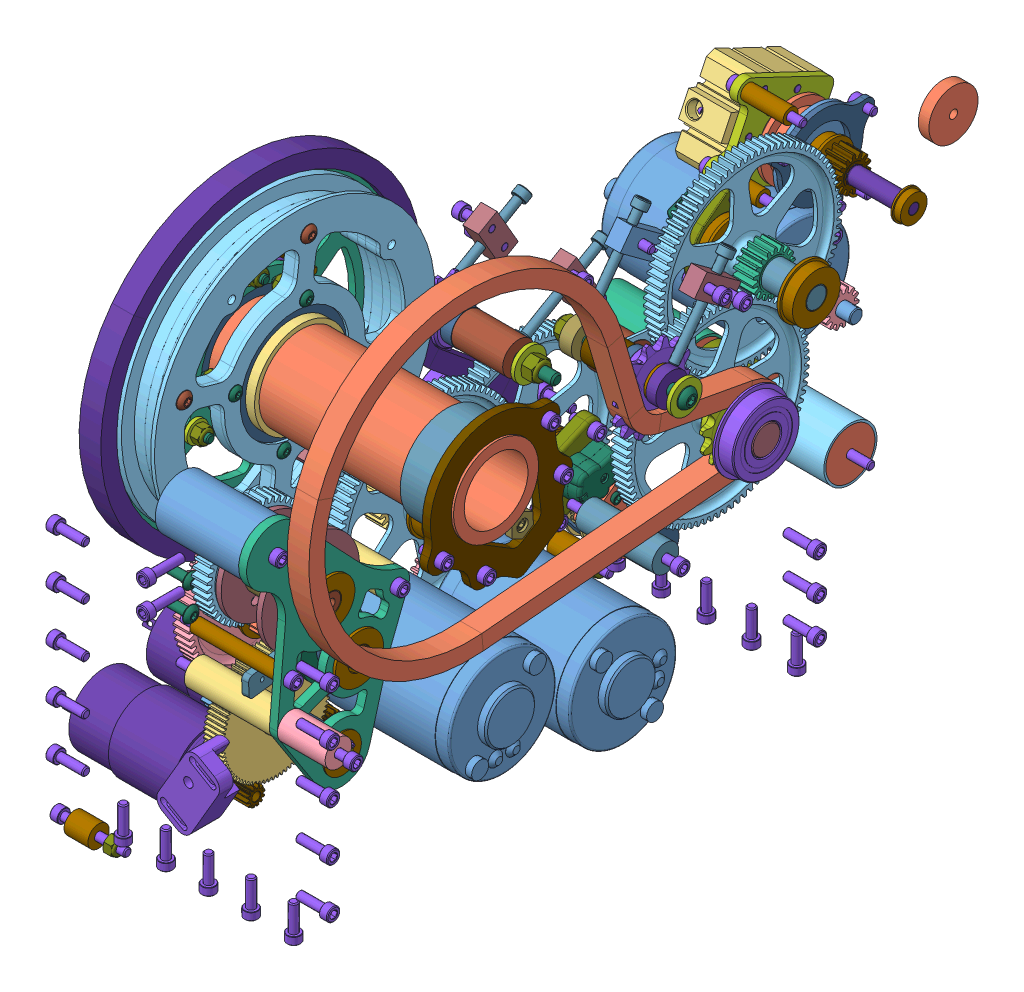
SolidWorks assembly 971-18-A-2900_Arm Gearbox, configuration Default. Lengths in mm. (continued)
Mates (geometry in assembly coordinates): (continued)
- Concentric136: concentric aligned: cylinder of 971-18-P-0057_Arm Gearbox Plates-1 through (0 -27.627 -17.6289) axis (-1 0 0) radius 2.0193; cylinder of 84865A130_10-32 Mitebite LOW-PROFILE CLAMP-1 through (-3.5814 -27.627 -17.6289) axis (-1 0 0) radius 2.413
- Coincident139: coincident anti-aligned: plane of 971-18-P-0057_Arm Gearbox Plates-1 through (0 0 0) normal (-1 0 0); plane of 84865A130_10-32 Mitebite LOW-PROFILE CLAMP-1 through (0 -35.3804 -18.2274) normal (1 0 0)
- Parallel1: parallel anti-aligned: plane of 971-18-P-0101_Tensioner Strap-1 through (-4.7625 -29.9915 -25.9171) normal (0 0.842996 0.537919); plane of 84865A130_10-32 Mitebite LOW-PROFILE CLAMP-1 through (-4.064 -31.4362 -24.4085) normal (0 -0.842996 -0.537919)
- Concentric137: concentric anti-aligned: cylinder of 971-18-P-0057_Arm Gearbox Plates-1 through (0 -27.627 -17.6289) axis (-1 0 0) radius 2.0193; cylinder of 84865A130_10-32 Mitebite LOW-PROFILE CLAMP-2 through (162.3314 -27.627 -17.6289) axis (1 0 0) radius 2.413
- Coincident141: coincident anti-aligned: plane of 971-18-P-0057_Arm Gearbox Plates-1 through (158.75 0 0) normal (1 0 0); plane of 84865A130_10-32 Mitebite LOW-PROFILE CLAMP-2 through (158.75 -31.4362 -24.4085) normal (-1 0 0)
- Parallel2: parallel anti-aligned: plane of 971-18-P-0101_Tensioner Strap-2 through (158.75 -29.9915 -25.9171) normal (0 0.842996 0.537919); plane of 84865A130_10-32 Mitebite LOW-PROFILE CLAMP-2 through (162.814 -35.3804 -18.2274) normal (0 -0.842996 -0.537919)
- Concentric138: concentric anti-aligned: cylinder of 971-18-P-0104_Arm Gearbox Proximal Arm Output Shaft-1 through (161.22 -58.42 -165.2367) axis (-1 0 0) radius 6.35; cylinder of 1_2in Shaft Collar, 217-2736-1 through (94.8323 -58.42 -165.2367) axis (1 0 0) radius 6.477
- Concentric140: concentric anti-aligned: cylinder of 971-18-P-0057_Arm Gearbox Plates-1 through (101.9302 42.553 -239.0191) axis (-1 0 0) radius 2.0193; cylinder of 971-18-A-4900_Brake Assembly-1/971-18-P-0165_Brake Piston Mount-1 through (71.628 42.553 -239.0191) axis (1 0 0) radius 6.35
- Concentric141: concentric aligned: cylinder of 971-18-P-0057_Arm Gearbox Plates-1 through (101.9302 24.3862 -284.3456) axis (-1 0 0) radius 2.0193; cylinder of 971-18-P-0148_Brake Pad-1 through (101.9302 24.3862 -284.3456) axis (-1 0 0) radius 2.4892
- Concentric142: concentric anti-aligned: cylinder of 971-18-P-0148_Brake Pad-1 through (101.9302 24.3862 -284.3456) axis (-1 0 0) radius 2.4892; cylinder of SHCS-2 through (98.7552 24.3862 -284.3456) axis (1 0 0) radius 2.413
- Coincident143: coincident anti-aligned: plane of 971-18-P-0148_Brake Pad-1 through (98.7552 27.1024 -246.9922) normal (-1 0 0); plane of SHCS-2 through (98.7552 28.0884 -283.9713) normal (1 0 0)
- Concentric143: concentric aligned: cylinder of 971-18-P-0057_Arm Gearbox Plates-1 through (106.6927 -24.2127 -256.9444) axis (1 0 0) radius 2.4892; cylinder of MiniCIM-1 through (101.9302 -24.2127 -256.9444) axis (1 0 0) radius 2.0193
- Coincident144: coincident anti-aligned: plane of 971-18-P-0057_Arm Gearbox Plates-1 through (106.6927 0 0) normal (1 0 0); plane of SHCS-5 through (106.6927 -23.145 -260.509) normal (-1 0 0)
- Concentric144: concentric anti-aligned: cylinder of 971-18-P-0057_Arm Gearbox Plates-1 through (106.6927 -24.2127 -256.9444) axis (1 0 0) radius 2.4892; cylinder of SHCS-5 through (106.6927 -24.2127 -256.9444) axis (-1 0 0) radius 2.413
- Concentric145: concentric anti-aligned: cylinder of 971-18-P-0057_Arm Gearbox Plates-1 through (106.6927 -66.0952 -228.1956) axis (1 0 0) radius 2.4892; cylinder of SHCS-6 through (106.6927 -66.0952 -228.1956) axis (-1 0 0) radius 2.413
- Coincident145: coincident anti-aligned: plane of 971-18-P-0057_Arm Gearbox Plates-1 through (106.6927 0 0) normal (1 0 0); plane of SHCS-6 through (106.6927 -65.0275 -231.7603) normal (-1 0 0)
- Concentric146: concentric aligned: cylinder of 971-18-P-0057_Arm Gearbox Plates-1 through (63.5 -146.0373 -33.9901) axis (-1 0 0) radius 2.4892; cylinder of MiniCIM-2 through (68.2625 -146.0373 -33.9901) axis (-1 0 0) radius 2.0193
- Concentric147: concentric aligned: cylinder of 971-18-P-0057_Arm Gearbox Plates-1 through (63.5 -164.4054 -67.0748) axis (-1 0 0) radius 2.4892; cylinder of MiniCIM-3 through (68.2625 -164.4054 -67.0748) axis (-1 0 0) radius 2.0193
- Coincident146: coincident anti-aligned: plane of 971-18-P-0057_Arm Gearbox Plates-1 through (63.5 0 0) normal (-1 0 0); plane of SHCS-7 through (63.5 -115.2256 2.9107) normal (1 0 0)
- Concentric148: concentric anti-aligned: cylinder of 971-18-P-0057_Arm Gearbox Plates-1 through (63.5 -111.5234 3.285) axis (-1 0 0) radius 2.4892; cylinder of SHCS-7 through (63.5 -111.5234 3.285) axis (1 0 0) radius 2.413
- Concentric149: concentric anti-aligned: cylinder of 971-18-P-0116_Arm Proximal Side Spacer-2 through (56.646 45.4322 -285.7008) axis (-1 0 0) radius 15.875; cylinder of 971-18-A-6600_Arm Hard Stop-1/971-18-P-0133_Arm hard stop-1 through (106.6927 45.4322 -285.7008) axis (1 0 0) radius 16.125
- Coincident147: coincident anti-aligned: plane of 971-18-P-0057_Arm Gearbox Plates-1 through (106.6927 0 0) normal (1 0 0); plane of 971-18-A-6600_Arm Hard Stop-1/971-18-P-0133_Arm hard stop-1 through (106.6927 68.5291 -272.3658) normal (-1 0 0)
- Angle1: planar angle = 0.523599 rad aligned: plane of 971-18-A-6600_Arm Hard Stop-1/971-18-P-0133_Arm hard stop-1 through (119.3927 68.5291 -272.3658) normal (0 -0.5 0.866025); plane of assembly through (0 0 0) normal (0 0 1)
- Coincident149: coincident anti-aligned: plane of 971-18-P-0057_Arm Gearbox Plates-1 through (152.4 0 0) normal (-1 0 0); plane of 971-18-P-0116_Arm Proximal Side Spacer-2 through (152.4 47.5844 -301.4292) normal (1 0 0)
- Concentric150: concentric aligned: cylinder of 971-18-P-0057_Arm Gearbox Plates-1 through (0 45.4322 -285.7008) axis (-1 0 0) radius 2.4892; cylinder of 971-18-P-0116_Arm Proximal Side Spacer-2 through (56.646 45.4322 -285.7008) axis (-1 0 0) radius 15.875
- Coincident150: coincident anti-aligned: plane of 971-18-P-0057_Arm Gearbox Plates-1 through (101.9302 0 0) normal (-1 0 0); plane of 971-18-P-0118_Arm Distal Side Double Spacer-1 through (101.9302 57.9871 -275.9854) normal (1 0 0)
- Concentric151: concentric aligned: cylinder of 971-18-P-0116_Arm Proximal Side Spacer-2 through (56.646 45.4322 -285.7008) axis (-1 0 0) radius 15.875; cylinder of 971-18-P-0118_Arm Distal Side Double Spacer-1 through (-18.7539 45.4322 -285.7008) axis (-1 0 0) radius 15.875
- Coincident151: coincident anti-aligned: plane of 971-18-P-0057_Arm Gearbox Plates-1 through (152.4 0 0) normal (-1 0 0); plane of 971-18-P-0116_Arm Proximal Side Spacer-1 through (152.4 -83.5681 -223.1773) normal (1 0 0)
- Concentric152: concentric aligned: cylinder of 971-18-P-0057_Arm Gearbox Plates-1 through (0 -99.4146 -224.1283) axis (-1 0 0) radius 2.4892; cylinder of 971-18-P-0116_Arm Proximal Side Spacer-1 through (56.646 -99.4146 -224.1283) axis (-1 0 0) radius 15.875
- Coincident152: coincident anti-aligned: plane of 971-18-P-0057_Arm Gearbox Plates-1 through (101.9302 0 0) normal (-1 0 0); plane of 971-18-P-0130_Arm Middle Spacer-1 through (101.9302 -100.3998 -239.9727) normal (1 0 0)
- Coincident153: coincident anti-aligned: plane of 971-18-P-0057_Arm Gearbox Plates-1 through (63.5 0 0) normal (-1 0 0); plane of 971-18-P-0115_Arm Distal Side Spacer-1 through (63.5 -85.5318 -216.4287) normal (1 0 0)
- Concentric153: concentric aligned: cylinder of 971-18-P-0057_Arm Gearbox Plates-1 through (0 -99.4146 -224.1283) axis (-1 0 0) radius 2.4892; cylinder of 971-18-P-0115_Arm Distal Side Spacer-1 through (-37.969 -99.4146 -224.1283) axis (-1 0 0) radius 15.875
- Concentric154: concentric aligned: cylinder of 971-18-P-0057_Arm Gearbox Plates-1 through (0 -166.289 -43.6572) axis (-1 0 0) radius 2.4892; cylinder of 971-18-P-0115_Arm Distal Side Spacer-2 through (-37.969 -166.289 -43.6572) axis (-1 0 0) radius 15.875
- Coincident154: coincident anti-aligned: plane of 971-18-P-0057_Arm Gearbox Plates-1 through (63.5 0 0) normal (-1 0 0); plane of 971-18-P-0115_Arm Distal Side Spacer-2 through (63.5 -173.1907 -29.361) normal (1 0 0)
- Concentric157: concentric anti-aligned: cylinder of 971-18-P-0057_Arm Gearbox Plates-1 through (101.9302 -98.1413 -113.6751) axis (-1 0 0) radius 2.4892; cylinder of 971-18-P-0185_Arm cross small standoff-1 through (153.5805 -98.1413 -113.6751) axis (1 0 0) radius 7.9375
- Coincident157: coincident anti-aligned: plane of 971-18-P-0057_Arm Gearbox Plates-1 through (106.6927 0 0) normal (1 0 0); plane of 971-18-P-0185_Arm cross small standoff-1 through (106.6927 -90.2038 -113.6751) normal (-1 0 0)
- Coincident158: coincident anti-aligned: plane of 3549S-1BA-102B-ND 10 turn potentiometer-1 through (66.775 -149.8585 -169.7731) normal (-1 0 0); plane of A-6z16-036df2508_36t plastic pulley-1 through (66.775 -149.8585 -169.7731) normal (1 0 0)
- Coincident166: coincident anti-aligned: plane of SRK Mag Encoder Magnet-2 through (107.2515 -2.1568 -197.4778) normal (1 0 0); plane of 971-18-P-0105_Arm Gearbox Proximal Arm First Stage Shaft -1 through (107.2515 -2.1568 -197.4778) normal (-1 0 0)
- Concentric1943: concentric aligned: cylinder of 971-18-P-0186_84T Gear With Access Hole-1 through (49.3125 -103.4997 -135.089) axis (-1 0 0) radius 8.89; cylinder of 971-18-P-0107_Arm Gearbox Distal Arm Output Shaft-1 through (69.8627 -103.4997 -135.089) axis (-1 0 0) radius 9.525
- Coincident214: coincident anti-aligned: plane of 971-18-P-0186_84T Gear With Access Hole-3 through (121.1339 -2.1568 -197.4778) normal (1 0 0); plane of 18T-1_2-Hex-Steel_217-5460-2 through (121.1339 -2.1568 -197.4778) normal (-1 0 0)
- Concentric1951: concentric anti-aligned: cylinder of 971-18-P-0116_Arm Proximal Side Spacer-1 through (56.646 -99.4146 -224.1283) axis (-1 0 0) radius 14.6304; cylinder of 971-18-P-0229_Arm Spacer Caps-1 through (100.1102 -99.4146 -224.1283) axis (1 0 0) radius 14.6685
- Coincident222: coincident aligned: plane of 971-18-P-0115_Arm Distal Side Spacer-1 through (6.35 -85.5318 -216.4287) normal (-1 0 0); plane of 971-18-P-0229_Arm Spacer Caps-1 through (6.35 -114.0127 -225.5645) normal (-1 0 0)
- Concentric1952: concentric anti-aligned: cylinder of 971-18-P-0116_Arm Proximal Side Spacer-1 through (56.646 -99.4146 -224.1283) axis (-1 0 0) radius 14.6304; cylinder of 971-18-P-0229_Arm Spacer Caps-7 through (150.9102 -99.4146 -224.1283) axis (1 0 0) radius 14.6685
- Coincident223: coincident aligned: plane of 971-18-P-0115_Arm Distal Side Spacer-1 through (63.5 -85.5318 -216.4287) normal (1 0 0); plane of 971-18-P-0229_Arm Spacer Caps-7 through (63.5 -86.8108 -216.6244) normal (1 0 0)
- Concentric1955: concentric anti-aligned: cylinder of 971-18-P-0130_Arm Middle Spacer-1 through (12.196 -99.4146 -224.1283) axis (-1 0 0) radius 14.6304; cylinder of 971-18-P-0229_Arm Spacer Caps-3 through (162.01 -99.4146 -224.1283) axis (1 0 0) radius 14.6685
- Coincident225: coincident aligned: plane of 971-18-P-0130_Arm Middle Spacer-1 through (68.2498 -100.3998 -239.9727) normal (-1 0 0); plane of 971-18-P-0229_Arm Spacer Caps-3 through (68.2498 -113.7159 -220.8666) normal (-1 0 0)
- Concentric1956: concentric aligned: cylinder of 971-18-P-0130_Arm Middle Spacer-1 through (12.196 -99.4146 -224.1283) axis (-1 0 0) radius 14.6304; cylinder of 971-18-P-0229_Arm Spacer Caps-5 through (8.17 -99.4146 -224.1283) axis (-1 0 0) radius 14.6685
- Coincident227: coincident aligned: plane of 971-18-P-0130_Arm Middle Spacer-1 through (101.9302 -100.3998 -239.9727) normal (1 0 0); plane of 971-18-P-0229_Arm Spacer Caps-5 through (101.9302 -84.7547 -224.6303) normal (1 0 0)
- Concentric1958: concentric anti-aligned: cylinder of 971-18-P-0116_Arm Proximal Side Spacer-1 through (56.646 -99.4146 -224.1283) axis (-1 0 0) radius 14.6304; cylinder of 971-18-P-0229_Arm Spacer Caps-2 through (200.4402 -99.4146 -224.1283) axis (1 0 0) radius 14.6685
- Coincident229: coincident aligned: plane of 971-18-P-0116_Arm Proximal Side Spacer-1 through (106.68 -83.5681 -223.1773) normal (-1 0 0); plane of 971-18-P-0229_Arm Spacer Caps-2 through (106.68 -114.0287 -222.8661) normal (-1 0 0)
- Coincident233: coincident aligned: plane of 971-18-P-0116_Arm Proximal Side Spacer-1 through (152.4 -83.5681 -223.1773) normal (1 0 0); plane of 971-18-P-0229_Arm Spacer Caps-6 through (152.4 -114.0831 -224.1283) normal (1 0 0)
- Concentric1962: concentric anti-aligned: cylinder of 971-18-P-0116_Arm Proximal Side Spacer-1 through (56.646 -99.4146 -224.1283) axis (-1 0 0) radius 14.6304; cylinder of 971-18-P-0229_Arm Spacer Caps-6 through (239.8102 -99.4146 -224.1283) axis (1 0 0) radius 14.6685
- Concentric1963: concentric anti-aligned: cylinder of 971-18-P-0115_Arm Distal Side Spacer-2 through (-37.969 -166.289 -43.6572) axis (-1 0 0) radius 14.6304; cylinder of 971-18-P-0229_Arm Spacer Caps-4 through (100.1102 -166.289 -43.6572) axis (1 0 0) radius 14.6685
- Coincident234: coincident aligned: plane of 971-18-P-0115_Arm Distal Side Spacer-2 through (6.35 -173.1907 -29.361) normal (-1 0 0); plane of 971-18-P-0229_Arm Spacer Caps-4 through (6.35 -179.1054 -50.7921) normal (-1 0 0)
- Concentric1964: concentric anti-aligned: cylinder of 971-18-P-0115_Arm Distal Side Spacer-2 through (-37.969 -166.289 -43.6572) axis (-1 0 0) radius 14.6304; cylinder of 971-18-P-0229_Arm Spacer Caps-8 through (150.9102 -166.289 -43.6572) axis (1 0 0) radius 14.6685
- Coincident235: coincident aligned: plane of 971-18-P-0115_Arm Distal Side Spacer-2 through (63.5 -173.1907 -29.361) normal (1 0 0); plane of 971-18-P-0229_Arm Spacer Caps-8 through (63.5 -180.9575 -43.6572) normal (1 0 0)
- Concentric1967: concentric anti-aligned: cylinder of 971-18-P-0057_Arm Gearbox Plates-1 through (0 45.4322 -285.7008) axis (-1 0 0) radius 2.4892; cylinder of SHCS-1 through (0 45.4322 -285.7008) axis (1 0 0) radius 2.413
- Coincident238: coincident anti-aligned: plane of 971-18-P-0057_Arm Gearbox Plates-1 through (0 0 0) normal (-1 0 0); plane of SHCS-1 through (0 42.6322 -283.2499) normal (1 0 0)
- Concentric1968: concentric anti-aligned: cylinder of 971-18-P-0116_Arm Proximal Side Spacer-2 through (56.646 45.4322 -285.7008) axis (-1 0 0) radius 14.6304; cylinder of 971-18-P-0229_Arm Spacer Caps-11 through (239.8102 45.4322 -285.7008) axis (1 0 0) radius 14.6685
- Coincident239: coincident anti-aligned: plane of 971-18-P-0057_Arm Gearbox Plates-1 through (152.4 0 0) normal (-1 0 0); plane of 971-18-P-0229_Arm Spacer Caps-11 through (152.4 30.7637 -285.7008) normal (1 0 0)
- Concentric1969: concentric aligned: cylinder of 971-18-P-0116_Arm Proximal Side Spacer-2 through (56.646 45.4322 -285.7008) axis (-1 0 0) radius 14.6304; cylinder of 971-18-P-0229_Arm Spacer Caps-12 through (19.2825 45.4322 -285.7008) axis (-1 0 0) radius 14.6685
- Coincident240: coincident anti-aligned: plane of 971-18-P-0057_Arm Gearbox Plates-1 through (106.6927 0 0) normal (1 0 0); plane of 971-18-P-0229_Arm Spacer Caps-12 through (106.6927 48.813 -299.9744) normal (-1 0 0)
- Concentric1970: concentric anti-aligned: cylinder of 971-18-P-0116_Arm Proximal Side Spacer-2 through (56.646 45.4322 -285.7008) axis (-1 0 0) radius 14.6304; cylinder of 971-18-P-0229_Arm Spacer Caps-13 through (189.3404 45.4322 -285.7008) axis (1 0 0) radius 14.6685
- Coincident241: coincident anti-aligned: plane of 971-18-P-0057_Arm Gearbox Plates-1 through (101.9302 0 0) normal (-1 0 0); plane of 971-18-P-0229_Arm Spacer Caps-13 through (101.9302 31.3632 -289.8518) normal (1 0 0)
- Concentric1971: concentric aligned: cylinder of 971-18-P-0116_Arm Proximal Side Spacer-2 through (56.646 45.4322 -285.7008) axis (-1 0 0) radius 14.6304; cylinder of 971-18-P-0229_Arm Spacer Caps-14 through (-81.0602 45.4322 -285.7008) axis (-1 0 0) radius 14.6685
- Coincident242: coincident anti-aligned: plane of 971-18-P-0057_Arm Gearbox Plates-1 through (6.35 0 0) normal (1 0 0); plane of 971-18-P-0229_Arm Spacer Caps-14 through (6.35 45.6015 -300.3683) normal (-1 0 0)
- Concentric1973: concentric anti-aligned: cylinder of 971-18-P-0057_Arm Gearbox Plates-1 through (0 -99.4146 -224.1283) axis (-1 0 0) radius 2.4892; cylinder of SHCS-13 through (0 -99.4146 -224.1283) axis (1 0 0) radius 2.413
- Coincident243: coincident anti-aligned: plane of 971-18-P-0057_Arm Gearbox Plates-1 through (0 0 0) normal (-1 0 0); plane of SHCS-13 through (0 -102.1778 -221.636) normal (1 0 0)
- Concentric1974: concentric anti-aligned: cylinder of 971-18-P-0057_Arm Gearbox Plates-1 through (0 -166.289 -43.6572) axis (-1 0 0) radius 2.4892; cylinder of SHCS-14 through (0 -166.289 -43.6572) axis (1 0 0) radius 2.413
- Coincident244: coincident anti-aligned: plane of 971-18-P-0057_Arm Gearbox Plates-1 through (0 0 0) normal (-1 0 0); plane of SHCS-14 through (0 -169.0522 -41.1649) normal (1 0 0)
- Concentric1975: concentric aligned: cylinder of 971-18-P-0057_Arm Gearbox Plates-1 through (101.9302 -98.1413 -113.6751) axis (-1 0 0) radius 2.4892; cylinder of SHCS-16 through (158.75 -98.1413 -113.6751) axis (-1 0 0) radius 2.413
- Coincident245: coincident anti-aligned: plane of 971-18-P-0057_Arm Gearbox Plates-1 through (158.75 0 0) normal (1 0 0); plane of SHCS-16 through (158.75 -97.4126 -117.3241) normal (-1 0 0)
- Concentric1979: concentric anti-aligned: cylinder of Bearings-5 through (98.4246 -2.1568 -197.4778) axis (-1 0 0) radius 14.2875; cylinder of 971-18-A-5400_SRX Mag Encoder 15 Assembly-1/971-18-P-0205_SRX Mag Encoder 15 Mount-3 through (99.7712 -2.1568 -197.4778) axis (1 0 0) radius 14.3002
- Coincident248: coincident anti-aligned: plane of 971-18-P-0057_Arm Gearbox Plates-1 through (101.9302 0 0) normal (-1 0 0); plane of 971-18-A-5400_SRX Mag Encoder 15 Assembly-1/971-18-P-0205_SRX Mag Encoder 15 Mount-3 through (101.9302 -2.1568 -197.4778) normal (1 0 0)
- Concentric1981: concentric anti-aligned: cylinder of 971-18-P-0057_Arm Gearbox Plates-1 through (101.9302 17.5344 -204.6448) axis (-1 0 0) radius 2.0193; cylinder of 971-18-A-5400_SRX Mag Encoder 15 Assembly-1/SHCS-2 through (93.9927 17.5344 -204.6448) axis (1 0 0) radius 2.413
- Concentric1982: concentric anti-aligned: cylinder of Bearings-1 through (71.7681 -103.4997 -135.089) axis (1 0 0) radius 14.2875; cylinder of 971-18-A-5400_SRX Mag Encoder 15 Assembly-2/971-18-P-0205_SRX Mag Encoder 15 Mount-3 through (70.4215 -103.4997 -135.089) axis (-1 0 0) radius 14.3002
- Coincident249: coincident anti-aligned: plane of 971-18-P-0057_Arm Gearbox Plates-1 through (68.2625 0 0) normal (1 0 0); plane of 971-18-A-5400_SRX Mag Encoder 15 Assembly-2/971-18-P-0205_SRX Mag Encoder 15 Mount-3 through (68.2625 -103.4997 -135.089) normal (-1 0 0)
- Concentric1983: concentric anti-aligned: cylinder of 971-18-P-0057_Arm Gearbox Plates-1 through (68.2625 -120.9185 -123.44) axis (1 0 0) radius 2.0193; cylinder of 971-18-A-5400_SRX Mag Encoder 15 Assembly-2/SHCS-1 through (76.2 -120.9185 -123.44) axis (-1 0 0) radius 2.413
- Concentric1984: concentric aligned: cylinder of 971-18-P-0101_Tensioner Strap-2 through (158.75 20.3652 -31.9152) axis (-1 0 0) radius 2.5527; cylinder of SHCS-19 through (163.5125 20.3652 -31.9152) axis (-1 0 0) radius 2.413
- Coincident250: coincident anti-aligned: plane of 971-18-P-0101_Tensioner Strap-2 through (163.5125 0 0) normal (1 0 0); plane of SHCS-19 through (163.5125 24.0861 -31.9561) normal (-1 0 0)
- Concentric1985: concentric anti-aligned: cylinder of 971-18-P-0101_Tensioner Strap-1 through (-4.7625 -20.3652 31.9152) axis (-1 0 0) radius 2.5527; cylinder of SHCS-23 through (-4.7625 -20.3652 31.9152) axis (1 0 0) radius 2.413
- Coincident252: coincident anti-aligned: plane of 971-18-P-0101_Tensioner Strap-1 through (-4.7625 0 0) normal (-1 0 0); plane of SHCS-23 through (-4.7625 -16.968 33.4336) normal (1 0 0)
- Concentric1988: concentric anti-aligned: cylinder of 971-18-P-0057_Arm Gearbox Plates-1 through (158.75 -172.339 95.6183) axis (1 0 0) radius 2.4892; cylinder of SHCS-27 through (158.75 -172.339 95.6183) axis (-1 0 0) radius 2.413
- Coincident255: coincident anti-aligned: plane of 971-18-P-0057_Arm Gearbox Plates-1 through (158.75 0 0) normal (1 0 0); plane of SHCS-27 through (158.75 -169.0333 93.9099) normal (-1 0 0)
- Concentric1989: concentric aligned: cylinder of 971-18-P-0057_Arm Gearbox Plates-1 through (158.75 -172.339 95.6183) axis (1 0 0) radius 2.4892; cylinder of SHCS-28 through (0 -172.339 95.6183) axis (1 0 0) radius 2.413
- Coincident256: coincident anti-aligned: plane of 971-18-P-0057_Arm Gearbox Plates-1 through (0 0 0) normal (-1 0 0); plane of SHCS-28 through (0 -169.5759 93.126) normal (1 0 0)
- Concentric1990: concentric anti-aligned: cylinder of 971-18-P-0057_Arm Gearbox Plates-1 through (158.75 -175.26 -195.2625) axis (1 0 0) radius 2.4892; cylinder of SHCS-37 through (158.75 -175.26 -195.2625) axis (-1 0 0) radius 2.413
- Coincident257: coincident anti-aligned: plane of 971-18-P-0057_Arm Gearbox Plates-1 through (158.75 0 0) normal (1 0 0); plane of SHCS-37 through (158.75 -171.9014 -196.8646) normal (-1 0 0)
- Concentric1991: concentric aligned: cylinder of 971-18-P-0057_Arm Gearbox Plates-1 through (158.75 -175.26 -195.2625) axis (1 0 0) radius 2.4892; cylinder of SHCS-38 through (0 -175.26 -195.2625) axis (1 0 0) radius 2.413
- Coincident258: coincident anti-aligned: plane of 971-18-P-0057_Arm Gearbox Plates-1 through (0 0 0) normal (-1 0 0); plane of SHCS-38 through (0 -172.4969 -197.7548) normal (1 0 0)
- Concentric1995: concentric anti-aligned: cylinder of 971-18-P-0057_Arm Gearbox Plates-1 through (139.6577 -188.214 95.6183) axis (0 -1 0) radius 2.0193; cylinder of SHCS-46 through (139.6577 -192.9892 95.6183) axis (0 1 0) radius 2.413
- Distance1: distance = 4.7752 mm anti-aligned: plane of 971-18-P-0057_Arm Gearbox Plates-1 through (152.4 -188.214 90.8558) normal (0 -1 0); plane of SHCS-46 through (143.3668 -192.9892 95.3205) normal (0 1 0)
- Concentric1996: concentric anti-aligned: cylinder of 971-18-P-0057_Arm Gearbox Plates-1 through (114.2153 -188.214 95.6183) axis (0 -1 0) radius 2.0193; cylinder of SHCS-47 through (114.2153 -192.9892 95.6183) axis (0 1 0) radius 2.413
- Coincident264: coincident aligned: plane of SHCS-46 through (143.3668 -192.9892 95.3205) normal (0 1 0); plane of SHCS-47 through (117.9245 -192.9892 95.3205) normal (0 1 0)
- Concentric1997: concentric anti-aligned: cylinder of 971-18-P-0057_Arm Gearbox Plates-1 through (88.773 -188.214 95.6183) axis (0 -1 0) radius 2.0193; cylinder of SHCS-48 through (88.773 -192.9892 95.6183) axis (0 1 0) radius 2.413
- Coincident265: coincident aligned: plane of SHCS-46 through (143.3668 -192.9892 95.3205) normal (0 1 0); plane of SHCS-48 through (92.3596 -192.9892 94.6268) normal (0 1 0)
- Coincident266: coincident aligned: plane of SHCS-46 through (143.3668 -192.9892 95.3205) normal (0 1 0); plane of SHCS-49 through (66.6192 -192.9892 93.8769) normal (0 1 0)
- Concentric1998: concentric anti-aligned: cylinder of 971-18-P-0057_Arm Gearbox Plates-1 through (63.3307 -188.214 95.6183) axis (0 -1 0) radius 2.0193; cylinder of SHCS-49 through (63.3307 -192.9892 95.6183) axis (0 1 0) radius 2.413
- Coincident267: coincident aligned: plane of SHCS-46 through (143.3668 -192.9892 95.3205) normal (0 1 0); plane of SHCS-50 through (40.677 -192.9892 93.1545) normal (0 1 0)
- Concentric1999: concentric anti-aligned: cylinder of 971-18-P-0057_Arm Gearbox Plates-1 through (37.8883 -188.214 95.6183) axis (0 -1 0) radius 2.0193; cylinder of SHCS-50 through (37.8883 -192.9892 95.6183) axis (0 1 0) radius 2.413
- Concentric2000: concentric anti-aligned: cylinder of 971-18-P-0057_Arm Gearbox Plates-1 through (122.2375 -190.5 -195.2625) axis (0 -1 0) radius 2.0193; cylinder of SHCS-52 through (122.2375 -194.437 -195.2625) axis (0 1 0) radius 2.413
- Distance2: distance = 3.937 mm anti-aligned: plane of 971-18-P-0057_Arm Gearbox Plates-1 through (152.4 -190.5 -200.025) normal (0 -1 0); plane of SHCS-52 through (125.9467 -194.437 -195.5603) normal (0 1 0)
- Concentric2001: concentric anti-aligned: cylinder of 971-18-P-0057_Arm Gearbox Plates-1 through (95.25 -190.5 -195.2625) axis (0 -1 0) radius 2.0193; cylinder of SHCS-53 through (95.25 -194.437 -195.2625) axis (0 1 0) radius 2.413
- Coincident270: coincident aligned: plane of SHCS-52 through (125.9467 -194.437 -195.5603) normal (0 1 0); plane of SHCS-53 through (98.9592 -194.437 -195.5603) normal (0 1 0)
- Coincident271: coincident aligned: plane of SHCS-52 through (125.9467 -194.437 -195.5603) normal (0 1 0); plane of SHCS-54 through (152.8116 -194.437 -196.254) normal (0 1 0)
- Concentric2002: concentric anti-aligned: cylinder of 971-18-P-0057_Arm Gearbox Plates-1 through (149.225 -190.5 -195.2625) axis (0 -1 0) radius 2.0193; cylinder of SHCS-54 through (149.225 -194.437 -195.2625) axis (0 1 0) radius 2.413
- Coincident272: coincident aligned: plane of SHCS-52 through (125.9467 -194.437 -195.5603) normal (0 1 0); plane of SHCS-55 through (71.551 -194.437 -197.0039) normal (0 1 0)
- Concentric2003: concentric anti-aligned: cylinder of 971-18-P-0057_Arm Gearbox Plates-1 through (68.2625 -190.5 -195.2625) axis (0 -1 0) radius 2.0193; cylinder of SHCS-55 through (68.2625 -194.437 -195.2625) axis (0 1 0) radius 2.413
- Coincident273: coincident aligned: plane of SHCS-52 through (125.9467 -194.437 -195.5603) normal (0 1 0); plane of SHCS-56 through (44.0636 -194.437 -197.7263) normal (0 1 0)
- Concentric2004: concentric anti-aligned: cylinder of 971-18-P-0057_Arm Gearbox Plates-1 through (41.275 -190.5 -195.2625) axis (0 -1 0) radius 2.0193; cylinder of SHCS-56 through (41.275 -194.437 -195.2625) axis (0 1 0) radius 2.413
- Coincident278: coincident anti-aligned: plane of 971-18-P-0057_Arm Gearbox Plates-1 through (0 0 0) normal (-1 0 0); plane of SHCS-61 through (0 -205.8981 -198.6843) normal (1 0 0)
- Concentric2009: concentric anti-aligned: cylinder of 971-18-P-0057_Arm Gearbox Plates-1 through (0 -204.4065 -195.2752) axis (-1 0 0) radius 2.4892; cylinder of SHCS-61 through (0 -204.4065 -195.2752) axis (1 0 0) radius 2.413
- Coincident284: coincident anti-aligned: plane of 971-18-P-0057_Arm Gearbox Plates-1 through (6.35 0 0) normal (1 0 0); plane of No 10 Aluminum Spacer-8 through (6.35 -203.0692 -189.0676) normal (-1 0 0)
- Concentric2016: concentric aligned: cylinder of SHCS-61 through (0 -204.4065 -195.2752) axis (1 0 0) radius 2.413; cylinder of No 10 Aluminum Spacer-8 through (56.9589 -204.4065 -195.2752) axis (1 0 0) radius 6.35
- Concentric2020: concentric aligned: cylinder of 971-18-P-0124_Sketchy Chain Tensioner-1 through (15.875 -12.5246 -146.6125) axis (1 0 0) radius 2.0193; cylinder of SHCS-65 through (0 -12.5246 -146.6125) axis (1 0 0) radius 2.413
- Concentric2021: concentric aligned: cylinder of 971-18-P-0124_Sketchy Chain Tensioner-1 through (15.875 -25.7229 -154.2325) axis (1 0 0) radius 2.0193; cylinder of SHCS-67 through (0 -25.7229 -154.2325) axis (1 0 0) radius 2.413
- Concentric2022: concentric aligned: cylinder of 971-18-P-0264_Swoopy thing 2-1 through (101.9302 21.0025 -150.0962) axis (1 0 0) radius 2.4892; cylinder of SHCS-69 through (92.4052 21.0025 -150.0962) axis (1 0 0) radius 2.413
- Coincident291: coincident anti-aligned: plane of 971-18-P-0264_Swoopy thing 2-1 through (92.4052 24.7667 -144.9822) normal (-1 0 0); plane of SHCS-69 through (92.4052 17.8262 -148.1577) normal (1 0 0)
- Concentric2023: concentric aligned: cylinder of 971-18-P-0264_Swoopy thing 2-1 through (101.9302 13.4742 -160.3243) axis (1 0 0) radius 2.4892; cylinder of SHCS-71 through (92.4052 13.4742 -160.3243) axis (1 0 0) radius 2.413
- Coincident292: coincident anti-aligned: plane of 971-18-P-0264_Swoopy thing 2-1 through (92.4052 24.7667 -144.9822) normal (-1 0 0); plane of SHCS-71 through (92.4052 10.2792 -158.4168) normal (1 0 0)
- Concentric2028: concentric aligned: cylinder of 3547S-1AA-102A-ND 3 Turn Potentiometer Bourns-2 through (90.4741 -58.42 -165.2367) axis (-1 0 0) radius 4.5; cylinder of 971-18-P-0243_Arm Gearbox Potentiometer Mount-2 through (101.9312 -58.42 -165.2367) axis (-1 0 0) radius 5.08
- Coincident296: coincident anti-aligned: plane of 971-18-P-0057_Arm Gearbox Plates-1 through (101.9302 0 0) normal (-1 0 0); plane of 971-18-P-0243_Arm Gearbox Potentiometer Mount-2 through (101.9302 -85.7984 -149.5368) normal (1 0 0)
- Parallel3: parallel aligned: plane of 971-18-P-0057_Arm Gearbox Plates-1 through (158.75 -117.7253 -222.1704) normal (0 -0.994332 0.106322); plane of 971-18-P-0243_Arm Gearbox Potentiometer Mount-2 through (100.4062 -73.1704 -150.8871) normal (0 -0.994332 0.106322)
- Concentric2029: concentric anti-aligned: cylinder of 971-18-P-0186_84T Gear With Access Hole-4 through (121.1339 -58.42 -165.2367) axis (1 0 0) radius 8.89; cylinder of VexPro_Hex Spacers-1 through (121.1339 -58.42 -165.2367) axis (-1 0 0) radius 9.7536
- Coincident297: coincident anti-aligned: plane of 971-18-P-0186_84T Gear With Access Hole-4 through (121.1339 -58.42 -165.2367) normal (-1 0 0); plane of VexPro_Hex Spacers-1 through (121.1339 -58.42 -165.2367) normal (1 0 0)
- Coincident298: coincident anti-aligned: plane of 971-18-P-0057_Arm Gearbox Plates-1 through (0 0 0) normal (-1 0 0); plane of SHCS-65 through (0 -14.681 -143.5799) normal (1 0 0)
- Coincident299: coincident anti-aligned: plane of 971-18-P-0057_Arm Gearbox Plates-1 through (0 0 0) normal (-1 0 0); plane of SHCS-67 through (0 -26.6968 -150.6411) normal (1 0 0)
- Concentric2030: concentric anti-aligned: cylinder of 971-18-P-0057_Arm Gearbox Plates-1 through (158.75 29.2837 -138.8453) axis (1 0 0) radius 2.4892; cylinder of SHCS-76 through (158.75 29.2837 -138.8453) axis (-1 0 0) radius 2.413
- Coincident300: coincident anti-aligned: plane of 971-18-P-0057_Arm Gearbox Plates-1 through (158.75 0 0) normal (1 0 0); plane of SHCS-76 through (158.75 32.7317 -140.2447) normal (-1 0 0)
- Concentric2031: concentric anti-aligned: cylinder of 971-18-P-0057_Arm Gearbox Plates-1 through (158.75 20.2497 -151.119) axis (1 0 0) radius 2.4892; cylinder of SHCS-78 through (158.75 20.2497 -151.119) axis (-1 0 0) radius 2.413
- Coincident301: coincident anti-aligned: plane of 971-18-P-0057_Arm Gearbox Plates-1 through (158.75 0 0) normal (1 0 0); plane of SHCS-78 through (158.75 23.4914 -152.946) normal (-1 0 0)
- Concentric2032: concentric aligned: cylinder of 971-18-P-0057_Arm Gearbox Plates-1 through (0 -12.5246 -146.6125) axis (-1 0 0) radius 2.4892; cylinder of SHCS-80 through (68.2625 -12.5246 -146.6125) axis (-1 0 0) radius 2.413
- Coincident302: coincident anti-aligned: plane of 971-18-P-0057_Arm Gearbox Plates-1 through (68.2625 0 0) normal (1 0 0); plane of SHCS-80 through (68.2625 -10.9765 -149.9963) normal (-1 0 0)
- Concentric2033: concentric aligned: cylinder of 971-18-P-0057_Arm Gearbox Plates-1 through (0 -25.7229 -154.2325) axis (-1 0 0) radius 2.4892; cylinder of SHCS-82 through (68.2625 -25.7229 -154.2325) axis (-1 0 0) radius 2.413
- Coincident303: coincident anti-aligned: plane of 971-18-P-0057_Arm Gearbox Plates-1 through (68.2625 0 0) normal (1 0 0); plane of SHCS-82 through (68.2625 -24.7858 -157.8337) normal (-1 0 0)
- Concentric2034: concentric aligned: cylinder of 971-18-P-0186_84T Gear With Access Hole-1 through (49.3125 -103.4997 -135.089) axis (-1 0 0) radius 8.89; cylinder of VexPro_Hex Spacers-2 through (61.9125 -103.4997 -135.089) axis (-1 0 0) radius 9.7536
- Coincident305: coincident anti-aligned: plane of SRK Mag Encoder Magnet-1 through (63.0047 -103.4997 -135.089) normal (-1 0 0); plane of 971-18-P-0107_Arm Gearbox Distal Arm Output Shaft-1 through (63.0047 -100.5783 -133.8458) normal (1 0 0)
- Coincident306: coincident anti-aligned: plane of Bearings-1 through (61.9125 -89.5132 -138.0061) normal (-1 0 0); plane of VexPro_Hex Spacers-2 through (61.9125 -103.4997 -135.089) normal (1 0 0)
- Concentric2035: concentric aligned: cylinder of 971-18-P-0107_Arm Gearbox Distal Arm Output Shaft-1 through (69.8627 -103.4997 -135.089) axis (-1 0 0) radius 9.525; cylinder of 971-18-P-0254_40T plastic pulley hex-1 through (60.9806 -103.4997 -135.089) axis (-1 0 0) radius 15.113
- Coincident307: coincident anti-aligned: plane of 971-18-P-0186_84T Gear With Access Hole-1 through (49.3125 -103.4997 -135.089) normal (1 0 0); plane of 971-18-P-0254_40T plastic pulley hex-1 through (49.3125 -103.4997 -135.089) normal (-1 0 0)
- Concentric2036: concentric aligned: cylinder of 971-18-P-0107_Arm Gearbox Distal Arm Output Shaft-1 through (69.8627 -103.4997 -135.089) axis (-1 0 0) radius 9.525; cylinder of 971-18-P-0249_Distal Shaft Spacer-1 through (36.4604 -103.4997 -135.089) axis (-1 0 0) radius 9.75
- Coincident308: coincident anti-aligned: plane of 12T_Hex_217-2662-2 through (26.5543 -103.4997 -135.089) normal (1 0 0); plane of 971-18-P-0249_Distal Shaft Spacer-1 through (26.5543 -103.4997 -135.089) normal (-1 0 0)
- Parallel4: parallel anti-aligned: plane of 971-18-P-0057_Arm Gearbox Plates-1 through (158.75 -118.7209 -182.2708) normal (0 -0.800703 -0.599061); plane of 971-18-P-0112_Arm Gearbox Distal Potentiometer Mount-1 through (68.345 -133.0932 -141.5671) normal (0 0.800703 0.599061)
- Parallel5: parallel aligned: plane of potentiometer belt-1 through (51.6937 -103.4997 -135.089) normal (0 0.599061 -0.800703); plane of 971-18-P-0112_Arm Gearbox Distal Potentiometer Mount-1 through (68.345 -118.0672 -161.6507) normal (0 0.599061 -0.800703)
- Coincident311: coincident anti-aligned: plane of 3549S-1BA-102B-ND 10 turn potentiometer-1 through (74.695 -149.8585 -169.7731) normal (-1 0 0); plane of 971-18-P-0112_Arm Gearbox Distal Potentiometer Mount-1 through (74.695 -149.8585 -169.7731) normal (1 0 0)
- Concentric2037: concentric anti-aligned: cylinder of SHCS-61 through (0 -204.4065 -195.2752) axis (1 0 0) radius 2.413; cylinder of Nylon-Insert Locknut-3 through (25.6032 -204.4065 -195.2752) axis (-1 0 0) radius 2.0828
- Distance3: distance = 7.0485 mm anti-aligned: plane of No 10 Aluminum Spacer-8 through (20.6375 -203.0692 -189.0676) normal (1 0 0); plane of Nylon-Insert Locknut-3 through (27.686 -199.3722 -195.5352) normal (-1 0 0)
- Concentric2038: concentric anti-aligned: cylinder of 971-18-P-0057_Arm Gearbox Plates-1 through (68.2625 -128.7803 -15.3525) axis (-1 0 0) radius 9.5631; cylinder of MiniCIM-2 through (68.2625 -128.7803 -15.3525) axis (1 0 0) radius 31.877
- Coincident321: coordinate: point of 971-18-P-0057_Arm Gearbox Plates-1; point of 971-18-A-5700_Winch Gearbox-1/971-18-P-0057_Arm Gearbox Plates-1
- Concentric2047: concentric anti-aligned: cylinder of 971-18-P-0057_Arm Gearbox Plates-1 through (63.5 -51.689 86.0933) axis (1 0 0) radius 2.0193; cylinder of BHCS-3 through (53.975 -51.689 86.0933) axis (-1 0 0) radius 2.413
- Coincident322: coincident anti-aligned: plane of 971-18-P-0057_Arm Gearbox Plates-1 through (68.2625 0 0) normal (1 0 0); plane of BHCS-3 through (68.2625 -48.6377 89.5151) normal (-1 0 0)
- Concentric2048: concentric anti-aligned: cylinder of 971-18-P-0057_Arm Gearbox Plates-1 through (63.5 -69.1515 86.0933) axis (1 0 0) radius 2.0193; cylinder of BHCS-4 through (53.975 -69.1515 86.0933) axis (-1 0 0) radius 2.413
- Coincident323: coincident anti-aligned: plane of 971-18-P-0057_Arm Gearbox Plates-1 through (68.2625 0 0) normal (1 0 0); plane of BHCS-4 through (68.2625 -66.1002 89.5151) normal (-1 0 0)
- Concentric2049: concentric anti-aligned: cylinder of 971-18-P-0057_Arm Gearbox Plates-1 through (58.7375 -46.9265 100.3808) axis (0 0 1) radius 2.4892; cylinder of SHCS-88 through (58.7375 -46.9265 100.3808) axis (0 0 -1) radius 2.413
- Concentric2050: concentric anti-aligned: cylinder of 971-18-P-0057_Arm Gearbox Plates-1 through (58.7375 -64.389 100.3808) axis (0 0 1) radius 2.4892; cylinder of SHCS-89 through (58.7375 -64.389 100.3808) axis (0 0 -1) radius 2.413
- Coincident324: coincident anti-aligned: plane of 971-18-P-0057_Arm Gearbox Plates-1 through (152.4 -188.214 100.3808) normal (0 0 1); plane of SHCS-89 through (56.2452 -61.6259 100.3808) normal (0 0 -1)
- Coincident325: coincident anti-aligned: plane of 971-18-P-0057_Arm Gearbox Plates-1 through (152.4 -188.214 100.3808) normal (0 0 1); plane of SHCS-88 through (56.2452 -44.1634 100.3808) normal (0 0 -1)
- Concentric2051: concentric aligned: cylinder of 971-18-P-0057_Arm Gearbox Plates-1 through (63.5 -134.8658 -152.2116) axis (-1 0 0) radius 2.0193; cylinder of BHCS-6 through (61.995 -134.8658 -152.2116) axis (-1 0 0) radius 2.413
- Coincident326: coincident anti-aligned: plane of 971-18-P-0112_Arm Gearbox Distal Potentiometer Mount-1 through (74.695 -149.8585 -169.7731) normal (1 0 0); plane of BHCS-6 through (74.695 -130.8701 -154.4598) normal (-1 0 0)
- Coincident327: coincident anti-aligned: plane of 971-18-P-0112_Arm Gearbox Distal Potentiometer Mount-1 through (74.695 -149.8585 -169.7731) normal (1 0 0); plane of BHCS-7 through (74.695 -124.4777 -161.9329) normal (-1 0 0)
- Concentric2052: concentric aligned: cylinder of 971-18-P-0057_Arm Gearbox Plates-1 through (63.5 -128.7793 -160.3468) axis (-1 0 0) radius 2.0193; cylinder of BHCS-7 through (61.995 -128.7793 -160.3468) axis (-1 0 0) radius 2.413
- Concentric2053: concentric anti-aligned: cylinder of BHCS-1 through (86.614 -39.637 -114.8895) axis (1 0 0) radius 3.175; cylinder of 91525A416_1-4 Oversized Washer-1 through (0 -39.637 -114.8895) axis (-1 0 0) radius 9.525
- Coincident329: coincident anti-aligned: plane of 971-18-P-0057_Arm Gearbox Plates-1 through (0 0 0) normal (-1 0 0); plane of 91525A416_1-4 Oversized Washer-1 through (0 -39.637 -114.8895) normal (1 0 0)
- Concentric2054: concentric aligned: cylinder of 971-18-P-0123_Distal Tensioner Short Spacer-1 through (31.8387 -39.637 -114.8895) axis (1 0 0) radius 3.2639; cylinder of BHCS-1 through (86.614 -39.637 -114.8895) axis (1 0 0) radius 3.175
- Coincident330: coincident anti-aligned: plane of BHCS-1 through (-2.286 -45.1869 -114.8895) normal (1 0 0); plane of 91525A416_1-4 Oversized Washer-1 through (-2.286 -39.637 -114.8895) normal (-1 0 0)
- Concentric2055: concentric anti-aligned: cylinder of BHCS-1 through (86.614 -39.637 -114.8895) axis (1 0 0) radius 3.175; cylinder of 91525A416_1-4 Oversized Washer-2 through (70.5485 -39.637 -114.8895) axis (-1 0 0) radius 3.5687
- Coincident331: coincident anti-aligned: plane of 971-18-P-0057_Arm Gearbox Plates-1 through (68.2625 0 0) normal (1 0 0); plane of 91525A416_1-4 Oversized Washer-2 through (68.2625 -39.637 -114.8895) normal (-1 0 0)
- Coincident332: coincident anti-aligned: plane of Nylon-Insert Locknut-1 through (70.5485 -46.0512 -115.0309) normal (-1 0 0); plane of 91525A416_1-4 Oversized Washer-2 through (70.5485 -39.637 -114.8895) normal (1 0 0)
- Coincident333: coincident anti-aligned: plane of Nylon-Insert Locknut-2 through (94.4372 -11.816 -111.0726) normal (1 0 0); plane of 971-18-P-0123_Distal Tensioner Short Spacer-3 through (94.4372 -5.8623 -110.7598) normal (-1 0 0)
- Concentric2056: concentric aligned: cylinder of BHCS-2 through (84.836 -12.6592 -117.4327) axis (-1 0 0) radius 3.175; cylinder of 91525A416_1-4 Oversized Washer-3 through (161.036 -12.6592 -117.4327) axis (-1 0 0) radius 9.525
- Coincident334: coincident anti-aligned: plane of 971-18-P-0057_Arm Gearbox Plates-1 through (158.75 0 0) normal (1 0 0); plane of 91525A416_1-4 Oversized Washer-3 through (158.75 -12.6592 -117.4327) normal (-1 0 0)
- Concentric2057: concentric anti-aligned: cylinder of 971-18-P-0248_Proximal Tensioner Short Spacer-2 through (171.1668 -12.6592 -117.4327) axis (1 0 0) radius 3.2639; cylinder of BHCS-2 through (84.836 -12.6592 -117.4327) axis (-1 0 0) radius 3.175
- Coincident335: coincident anti-aligned: plane of BHCS-2 through (161.036 -14.7784 -112.3034) normal (-1 0 0); plane of 91525A416_1-4 Oversized Washer-3 through (161.036 -12.6592 -117.4327) normal (1 0 0)
- Coincident336: coincident anti-aligned: plane of SHCS-32 through (163.576 -50.5026 94.0207) normal (1 0 0); plane of 971-18-P-0057_Arm Gearbox Plates-2 through (163.576 -162.56 -197.485) normal (-1 0 0)
- Coincident337: coincident aligned: plane of 971-18-P-0057_Arm Gearbox Plates-1 through (158.75 -188.214 103.5558) normal (0 0 1); plane of 971-18-P-0057_Arm Gearbox Plates-2 through (164.3888 -162.56 103.5558) normal (0 0 1)
- Coincident338: coincident aligned: plane of 971-18-P-0057_Arm Gearbox Plates-1 through (158.75 25.8839 -19.8529) normal (0 0.983523 0.180782); plane of 971-18-P-0057_Arm Gearbox Plates-2 through (164.3888 28.6009 -34.6344) normal (0 0.983523 0.180782)
- Coincident339: coincident aligned: plane of 971-18-P-0057_Arm Gearbox Plates-1 through (158.75 -52.6379 -288.3169) normal (0 -0.161448 -0.986881); plane of 971-18-P-0057_Arm Gearbox Plates-3 through (-5.6388 42.4591 -303.8742) normal (0 -0.161448 -0.986881)
- Coincident340: coincident aligned: plane of 971-18-P-0057_Arm Gearbox Plates-1 through (158.75 25.8839 -19.8529) normal (0 0.989859 0.142055); plane of 971-18-P-0057_Arm Gearbox Plates-3 through (-5.6388 27.324 -29.8876) normal (0 0.989859 0.142055)
- Coincident341: coincident anti-aligned: plane of SHCS-1 through (-4.826 42.8138 -283.4088) normal (-1 0 0); plane of 971-18-P-0057_Arm Gearbox Plates-3 through (-4.826 0 0) normal (1 0 0)
- Coincident344: coincident anti-aligned: plane of 971-18-P-0057_Arm Gearbox Plates-1 through (152.4 -188.214 100.3808) normal (0 0 1); plane of 971-18-P-0352_Arm Gearbox-Bumper Spacer-1 through (90.8758 -115.2621 100.3808) normal (0 0 -1)
- Concentric2061: concentric anti-aligned: cylinder of 971-18-P-0057_Arm Gearbox Plates-1 through (89.6747 -134.4041 100.3808) axis (0 0 1) radius 2.0193; cylinder of 971-18-P-0352_Arm Gearbox-Bumper Spacer-1 through (89.6747 -134.4041 100.3808) axis (0 0 -1) radius 2.8067
